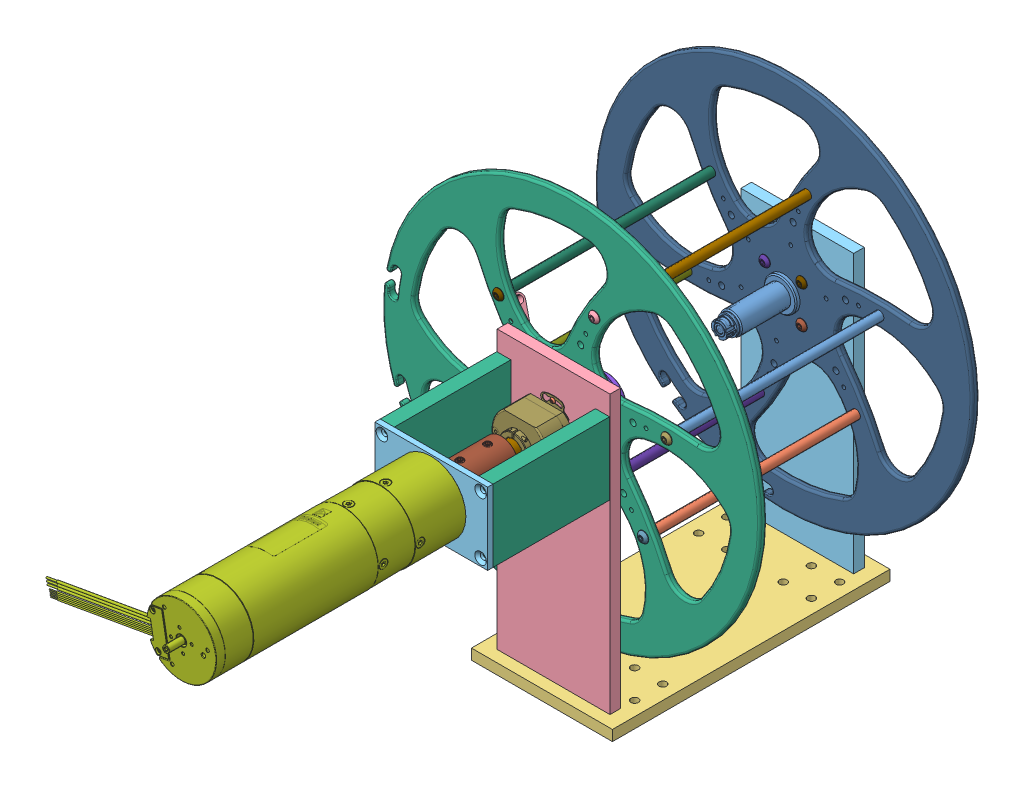
SolidWorks assembly MHK_PTO  v13 - Import, configuration Default. Lengths in mm.
Overall size (340 379.53 598.17).
53 component instances, 48 part files, 0 mates.
Components (placement in the parent):
- Spool Support.step-1: Spool Support.step [Default] at (-13.1975 -9.525 242.4976) x (0 0 -1) z (1 0 0) size (250 259.52 127)
  - 5448T18.step-1: 5448T18.step [Default] at (-67.0274 209.525 13.1975) x (0 -1 0) z (0 0 1) size (23 16 23)
  - 92095A113.step-1: 92095A113.step [Default] at (-66.9844 229.525 13.1975) x (0 0 -1) z (-1 0 0) size (4.5 4.5 4.5)
  - 92095A113.step-2: 92095A113.step [Default] at (-66.9844 189.525 13.1975) x (0 0 -1) z (-1 0 0) size (4.5 4.5 4.5)
  - Spool Support-0.step-1: Spool Support-0.step [Default] at origin size (250 9.53 127)
  - Spool Support-1.step-1: Spool Support-1.step [Default] at origin size (9.53 250 101.6)
  - Spool Support-2.step-1: Spool Support-2.step [Default] at origin size (9.53 250 101.6)
- Spool Core.step-1: Spool Core.step [Default] at (13.4446 195.1511 -46.5574) x (0 1 0) z (0 0 1) size (340 340 240.83)
  - Component12.step-1: Component12.step [Default] at (-7.5076 6.2623 2.175) x (0.766044 -0.642788 0) z (0 0 1) size (9.5 9.5 14.75)
  - Component13.step-1: Component13.step [Default] at (-7.5076 6.2623 2.175) x (0.766044 -0.642788 0) z (0 0 1) size (9.5 9.5 14.75)
  - Component14.step-1: Component14.step [Default] at (-10.8225 46.1728 670.1648) x (1 0 0) z (0 0 -1) size (9.5 9.5 14.75)
  - Component15.step-1: Component15.step [Default] at (-7.5076 6.2623 2.175) x (0.766044 -0.642788 0) z (0 0 1) size (9.5 9.5 14.75)
  - Spool Core-3.step-1: Spool Core-3.step [Default] at origin size (340 340 6.35)
  - Spool Core-4.step-1: Spool Core-4.step [Default] at origin size (9.5 9.5 14.75)
  - Spool Core-5.step-1: Spool Core-5.step [Default] at origin size (8.18 8.18 9.12)
  - Spool Core-6.step-1: Spool Core-6.step [Default] at origin size (9.5 9.5 14.75)
  - Spool Core-7.step-1: Spool Core-7.step [Default] at origin size (9.5 9.5 14.75)
  - Spool Core-8.step-1: Spool Core-8.step [Default] at origin size (8 8 185)
  - Spool Core-9.step-1: Spool Core-9.step [Default] at origin size (8 8 185)
  - Spool Core-10.step-1: Spool Core-10.step [Default] at origin size (8 8 185)
  - Spool Core-11.step-1: Spool Core-11.step [Default] at origin size (9.5 9.5 14.75)
  - Spool Core-12.step-1: Spool Core-12.step [Default] at origin size (8 8 185)
  - Spool Core-13.step-1: Spool Core-13.step [Default] at origin size (8 8 185)
  - Spool Core-14.step-1: Spool Core-14.step [Default] at origin size (9.5 9.5 14.75)
  - Spool Core-15.step-1: Spool Core-15.step [Default] at origin size (9.5 9.5 14.75)
  - Spool Core-16.step-1: Spool Core-16.step [Default] at origin size (9.5 9.5 14.75)
  - Spool Core-17.step-1: Spool Core-17.step [Default] at origin size (340 340 6.35)
  - Spool Core-18.step-1: Spool Core-18.step [Default] at origin size (17.75 23.28 7.94)
  - Spool Core-19.step-1: Spool Core-19.step [Default] at origin size (9.5 9.5 14.75)
  - Spool Core-20.step-1: Spool Core-20.step [Default] at origin size (8 8 185)
  - Spool Core-21.step-1: Spool Core-21.step [Default] at origin size (23.39 18.02 7.94)
  - Spool Core-22.step-1: Spool Core-22.step [Default] at origin size (9.5 9.5 14.75)
  - Spool Core-23.step-1: Spool Core-23.step [Default] at origin size (9.5 9.5 14.75)
  - Spool Core-24.step-1: Spool Core-24.step [Default] at origin size (9.5 9.5 14.75)
  - Spool Core-25.step-1: Spool Core-25.step [Default] at origin size (9.5 9.5 14.75)
  - Spool Core-26.step-1: Spool Core-26.step [Default] at origin size (8.18 8.18 9.12)
  - Spool Core-27.step-1: Spool Core-27.step [Default] at origin size (9.5 9.5 14.75)
  - Spool Core-28.step-1: Spool Core-28.step [Default] at origin size (9.5 9.5 14.75)
  - Spool Core-29.step-1: Spool Core-29.step [Default] at origin size (9.5 9.5 14.75)
  - Spool Core-30.step-1: Spool Core-30.step [Default] at origin size (56 56 99.65)
  - Spool Core-31.step-1: Spool Core-31.step [Default] at origin size (8.18 8.18 9.12)
  - Spool Core-32.step-1: Spool Core-32.step [Default] at origin size (9.5 9.5 14.75)
  - Spool Core-33.step-1: Spool Core-33.step [Default] at origin size (23.71 23.42 7.94)
- Motor Support.step-1: Motor Support.step [Default] at (-17.8977 208.142 457.889) x (0 0 1) z (-1 0 0) size (109.83 65 101.6)
  - Component1.step-1: Component1.step [Default] at (-45 0 0) size (4.83 65 101.6)
  - Component2.step-1: Component2.step [Default] at (-7.2906 1.3024 20.2023) size (105 65 12.7)
  - Component2.step-2: Component2.step [Default] at (-7.2906 1.3024 -68.6977) size (105 65 12.7)
- DC Motor.step-1: DC Motor.step [Default] at (0 200 412.715) x (0 0 1) z (0 1 0) size (278.16 164.16 78.2)
- Shaft Clamp.step-1: Shaft Clamp.step [Default] at (0 200 279.85) x (0.707107 0.707107 0) z (0 0 1) size (63 63 21)
- Shaft.step-1: Shaft.step [Default] at (0 200 272.525) size (16 16 118.4)
- Shaft Clamp Adapter.step-1: Shaft Clamp Adapter.step [Default] at (0 200 285.35) x (0 0 -1) z (0.707107 0.707107 0) size (6.35 68 68)
- Shaft Coupler.step-1: Shaft Coupler.step [Default] at (0 200 379.525) size (31 31.76 50.01)
- Encoder.step-1: Encoder.step [Default] at (0 200 319.36) x (1 0 0) z (0 0 -1) size (50.8 52.34 36.53)
